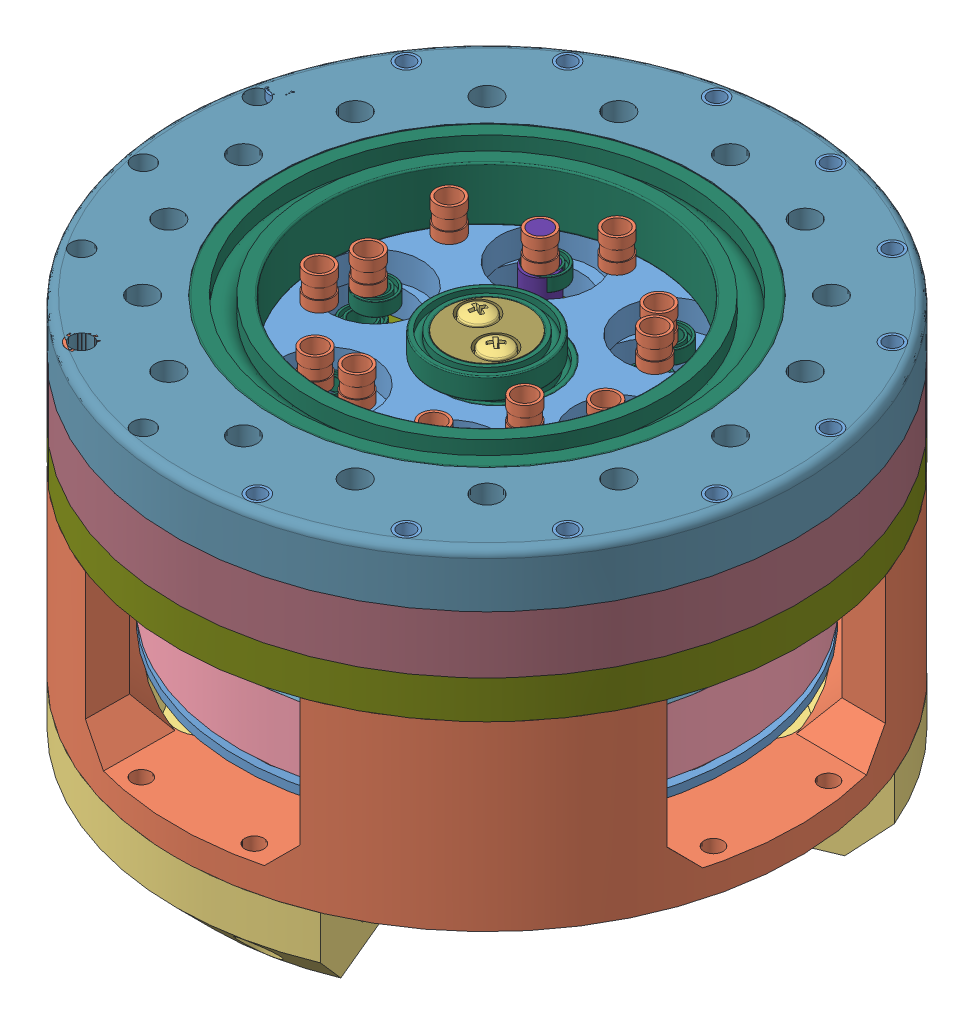
SolidWorks assembly Cycloidal, configuration Default. Lengths in mm. (continued)
Components (placement in the parent): (continued)
- hex nut style 1 gradeab_iso-1: hex nut style 1 gradeab_iso [ISO - 4032 - M3 - W - N] at (47.543 33.6573 58.7543) x (1 0 0) z (0 -1 0) size (5.5 6.35 2.4)
- Cycloidal_Discs_8308-1: Cycloidal_Discs_8308 [Default] at (106.6366 42.127 50.4062) x (-0.015094 0 0.999886) z (-0.999886 0 -0.015094) size (79.25 5 79.73)
  - Cycloidal_Discs-1: Cycloidal_Discs [Default] at (38.3081 39.5303 58.0959) size (79.25 5 79.73)
  - radial ball bearing_68_iso-1: radial ball bearing_68_iso [ISO 15 RBB - 274 - 14,SI,NC,14_68] at (18.3896 43.2803 46.5959) x (0 1 0) z (0 0 1) size (2.5 7 7)
  - radial ball bearing_68_iso-2: radial ball bearing_68_iso [ISO 15 RBB - 274 - 14,SI,NC,14_68] at (38.3081 43.2803 81.0959) x (0 1 0) z (0 0 1) size (2.5 7 7)
  - radial ball bearing_68_iso-3: radial ball bearing_68_iso [ISO 15 RBB - 274 - 14,SI,NC,14_68] at (18.3896 43.2803 69.5959) x (0 1 0) z (0 0 1) size (2.5 7 7)
  - radial ball bearing_68_iso-4: radial ball bearing_68_iso [ISO 15 RBB - 274 - 14,SI,NC,14_68] at (38.3081 43.2803 35.0959) x (0 1 0) z (0 0 1) size (2.5 7 7)
  - radial ball bearing_68_iso-5: radial ball bearing_68_iso [ISO 15 RBB - 274 - 14,SI,NC,14_68] at (58.2267 43.2803 69.5959) x (0 1 0) z (0 0 1) size (2.5 7 7)
  - radial ball bearing_68_iso-6: radial ball bearing_68_iso [ISO 15 RBB - 274 - 14,SI,NC,14_68] at (58.2267 43.2803 46.5959) x (0 1 0) z (0 0 1) size (2.5 7 7)
- Cycloidal_Discs_8308-2: Cycloidal_Discs_8308 [Default] at (106.2008 37.127 126.3479) x (-0.902001 0 0.431733) z (-0.431733 0 -0.902001) size (79.25 5 79.73)
  - Cycloidal_Discs-1: Cycloidal_Discs [Default] at (38.3081 39.5303 58.0959) size (79.25 5 79.73)
  - radial ball bearing_68_iso-1: radial ball bearing_68_iso [ISO 15 RBB - 274 - 14,SI,NC,14_68] at (18.3896 43.2803 46.5959) x (0 1 0) z (0 0 1) size (2.5 7 7)
  - radial ball bearing_68_iso-2: radial ball bearing_68_iso [ISO 15 RBB - 274 - 14,SI,NC,14_68] at (38.3081 43.2803 81.0959) x (0 1 0) z (0 0 1) size (2.5 7 7)
  - radial ball bearing_68_iso-3: radial ball bearing_68_iso [ISO 15 RBB - 274 - 14,SI,NC,14_68] at (18.3896 43.2803 69.5959) x (0 1 0) z (0 0 1) size (2.5 7 7)
  - radial ball bearing_68_iso-4: radial ball bearing_68_iso [ISO 15 RBB - 274 - 14,SI,NC,14_68] at (38.3081 43.2803 35.0959) x (0 1 0) z (0 0 1) size (2.5 7 7)
  - radial ball bearing_68_iso-5: radial ball bearing_68_iso [ISO 15 RBB - 274 - 14,SI,NC,14_68] at (58.2267 43.2803 69.5959) x (0 1 0) z (0 0 1) size (2.5 7 7)
  - radial ball bearing_68_iso-6: radial ball bearing_68_iso [ISO 15 RBB - 274 - 14,SI,NC,14_68] at (58.2267 43.2803 46.5959) x (0 1 0) z (0 0 1) size (2.5 7 7)
- m6-1: m6 [Default] at (36.6817 92.633 68.7393) x (0 0 -1) z (-1 0 0) size (6 16 6)
- Motor_Cover_v2-2: Motor_Cover_v2 [Default] at (47.267 36.0573 89.1587) x (0.999959 0 0.009078) z (-0.009078 0 0.999959) size (115 33.6 115)
- driver_cover-1: driver_cover [Default] at (47.267 36.0573 89.1587) x (0.925706 0 0.378243) z (0.378243 0 -0.925706) size (81.32 15 115)
Mates (geometry in assembly coordinates):
- Coincident1: coincident anti-aligned: plane of motor-X83008S.stp-1/outrunner.stp-1 through (63.4159 69.6573 58.6716) normal (0 1 0); plane of Base_Plate-1 through (47.267 69.6573 89.1587) normal (0 -1 0)
- Concentric1: concentric anti-aligned: line of motor-X83008S.stp-1/outrunner.stp-1 through (54.5223 64.1573 75.4616) axis (0 1 0); cylinder of Base_Plate-1 through (54.5223 76.6573 75.4616) axis (0 -1 0) radius 1.5
- Concentric2: concentric anti-aligned: cylinder of motor-X83008S.stp-1/shaft.stp-1 through (47.267 69.6573 89.1587) axis (0 1 0) radius 1.5; line of Base_Plate-1 through (47.267 76.6573 89.1587) axis (0 -1 0)
- Coincident2: coincident anti-aligned: plane of Base_Plate-1 through (47.267 76.6573 89.1587) normal (0 1 0); plane of Eccentric_Shaft-1/Eccentric_Shaft_bot-1 through (46.5649 76.6573 90.4842) normal (0 -1 0)
- Concentric75: concentric anti-aligned: cylinder of Output_Shaft-1 through (47.267 97.2573 89.1587) axis (0 -1 0) radius 30; cylinder of radial ball bearing_68_iso-39 through (47.267 71.6198 89.1587) axis (0 1 0) radius 30
- Concentric76: concentric anti-aligned: cylinder of Cover-1 through (47.267 97.2573 89.1587) axis (0 -1 0) radius 39; cylinder of radial ball bearing_68_iso-39 through (47.267 71.6198 89.1587) axis (0 1 0) radius 39
- Coincident104: coincident aligned: plane of Cover-1 through (47.267 97.2573 89.1587) normal (0 1 0); plane of radial ball bearing_68_iso-39 through (8.567 97.2573 89.1587) normal (0 1 0)
- Coincident105: coincident aligned: plane of Output_Shaft-1 through (47.267 97.2573 89.1587) normal (0 1 0); plane of Cover-1 through (47.267 97.2573 89.1587) normal (0 1 0)
- Concentric78: concentric anti-aligned: cylinder of Base_Plate-1 through (47.267 76.6573 89.1587) axis (0 -1 0) radius 20; cylinder of radial ball bearing_68_iso-40 through (47.267 52.3198 89.1587) axis (0 1 0) radius 20
- Concentric79: concentric aligned: cylinder of Ring_Pin_Housing-1 through (2.3676 87.2573 59.1579) axis (0 -1 0) radius 1.6; cylinder of Base_plate_2-1 through (2.3676 76.6573 59.1579) axis (0 -1 0) radius 1.75
- Concentric80: concentric aligned: cylinder of Ring_Pin_Housing-1 through (47.267 87.2573 89.1587) axis (0 -1 0) radius 57.5; cylinder of Base_plate_2-1 through (47.267 76.6573 89.1587) axis (0 -1 0) radius 57.5
- Coincident107: coincident anti-aligned: plane of Ring_Pin_Housing-1 through (47.267 76.6573 89.1587) normal (0 -1 0); plane of Base_plate_2-1 through (47.267 76.6573 89.1587) normal (0 1 0)
- Concentric83: concentric aligned: cylinder of Ring_Pin_Housing-1 through (2.3676 87.2573 59.1579) axis (0 -1 0) radius 1.6; cylinder of Cover-1 through (2.3676 97.2573 59.1579) axis (0 -1 0) radius 2
- Concentric84: concentric aligned: cylinder of Cover-1 through (15.4472 87.2573 57.3389) axis (0 1 0) radius 2.5; cylinder of m13_bearing-1/m6-1 through (15.4472 86.8573 57.3389) axis (0 1 0) radius 2
- Concentric85: concentric aligned: cylinder of Cover-1 through (47.267 87.2573 134.1587) axis (0 1 0) radius 2.5; cylinder of m13_bearing-11/m6-1 through (47.267 86.8573 134.1587) axis (0 1 0) radius 2
- Concentric86: concentric aligned: cylinder of Cover-1 through (64.4877 87.2573 130.7332) axis (0 1 0) radius 2.5; cylinder of m13_bearing-2/m6-1 through (64.4877 86.8573 130.7332) axis (0 1 0) radius 2
- Concentric87: concentric aligned: cylinder of Cover-1 through (79.0868 87.2573 120.9785) axis (0 1 0) radius 2.5; cylinder of m13_bearing-12/m6-1 through (79.0868 86.8573 120.9785) axis (0 1 0) radius 2
- Concentric88: concentric aligned: cylinder of Cover-1 through (88.8416 87.2573 106.3794) axis (0 1 0) radius 2.5; cylinder of m13_bearing-5/m6-1 through (88.8416 86.8573 106.3794) axis (0 1 0) radius 2
- Concentric89: concentric aligned: cylinder of Cover-1 through (92.267 87.2573 89.1587) axis (0 1 0) radius 2.5; cylinder of m13_bearing-4/m6-1 through (92.267 86.8573 89.1587) axis (0 1 0) radius 2
- Concentric90: concentric aligned: cylinder of Cover-1 through (30.0462 87.2573 47.5841) axis (0 1 0) radius 2.5; cylinder of m13_bearing-6/m6-1 through (30.0462 86.8573 47.5841) axis (0 1 0) radius 2
- Concentric91: concentric aligned: cylinder of Cover-1 through (47.267 87.2573 44.1587) axis (0 1 0) radius 2.5; cylinder of m13_bearing-3/m6-1 through (47.267 86.8573 44.1587) axis (0 1 0) radius 2
- Concentric92: concentric aligned: cylinder of Cover-1 through (64.4877 87.2573 47.5841) axis (0 1 0) radius 2.5; cylinder of m13_bearing-7/m6-1 through (64.4877 86.8573 47.5841) axis (0 1 0) radius 2
- Concentric93: concentric aligned: cylinder of Cover-1 through (79.0868 87.2573 57.3389) axis (0 1 0) radius 2.5; cylinder of m13_bearing-8/m6-1 through (79.0868 86.8573 57.3389) axis (0 1 0) radius 2
- Concentric94: concentric aligned: cylinder of Cover-1 through (88.8416 87.2573 71.9379) axis (0 1 0) radius 2.5; cylinder of m13_bearing-9/m6-1 through (88.8416 86.8573 71.9379) axis (0 1 0) radius 2
- Concentric96: concentric aligned: cylinder of Base_plate_2-1 through (47.267 76.6573 134.1587) axis (0 -1 0) radius 2.5; cylinder of socket button head screw_iso-2 through (47.267 67.4573 134.1587) axis (0 -1 0) radius 2
- Coincident121: coincident anti-aligned: plane of Base_plate_2-1 through (47.267 69.6573 89.1587) normal (0 -1 0); plane of socket button head screw_iso-2 through (45.8877 69.6573 132.7104) normal (0 1 0)
- Concentric971: concentric aligned: cylinder of Base_plate_2-1 through (15.4472 76.6573 57.3389) axis (0 -1 0) radius 2.5; cylinder of socket button head screw_iso-3 through (15.4472 67.4573 57.3389) axis (0 -1 0) radius 3.8
- Coincident1221: coincident anti-aligned: plane of Base_plate_2-1 through (47.267 69.6573 89.1587) normal (0 -1 0); plane of socket button head screw_iso-3 through (14.0679 69.6573 55.8906) normal (0 1 0)
- Concentric981: concentric aligned: cylinder of Base_plate_2-1 through (30.0462 76.6573 47.5841) axis (0 -1 0) radius 2.5; cylinder of socket button head screw_iso-4 through (30.0462 67.4573 47.5841) axis (0 -1 0) radius 3.8
- Coincident1231: coincident anti-aligned: plane of Base_plate_2-1 through (47.267 69.6573 89.1587) normal (0 -1 0); plane of socket button head screw_iso-4 through (28.6669 69.6573 46.1358) normal (0 1 0)
- Concentric991: concentric aligned: cylinder of Base_plate_2-1 through (47.267 76.6573 44.1587) axis (0 -1 0) radius 2.5; cylinder of socket button head screw_iso-5 through (47.267 67.4573 44.1587) axis (0 -1 0) radius 3.8
- Coincident1241: coincident anti-aligned: plane of Base_plate_2-1 through (47.267 69.6573 89.1587) normal (0 -1 0); plane of socket button head screw_iso-5 through (45.8877 69.6573 42.7104) normal (0 1 0)
- Concentric1001: concentric aligned: cylinder of Base_plate_2-1 through (64.4877 76.6573 47.5841) axis (0 -1 0) radius 2.5; cylinder of socket button head screw_iso-6 through (64.4877 67.4573 47.5841) axis (0 -1 0) radius 3.8
- Coincident1251: coincident anti-aligned: plane of Base_plate_2-1 through (47.267 69.6573 89.1587) normal (0 -1 0); plane of socket button head screw_iso-6 through (63.1085 69.6573 46.1358) normal (0 1 0)
- Concentric1021: concentric aligned: cylinder of Base_plate_2-1 through (88.8416 76.6573 71.9379) axis (0 -1 0) radius 2.5; cylinder of socket button head screw_iso-8 through (88.8416 67.4573 71.9379) axis (0 -1 0) radius 3.8
- Coincident1271: coincident anti-aligned: plane of Base_plate_2-1 through (47.267 69.6573 89.1587) normal (0 -1 0); plane of socket button head screw_iso-8 through (87.4623 69.6573 70.4896) normal (0 1 0)
- Concentric1031: concentric aligned: cylinder of Base_plate_2-1 through (92.267 76.6573 89.1587) axis (0 -1 0) radius 2.5; cylinder of socket button head screw_iso-9 through (92.267 67.4573 89.1587) axis (0 -1 0) radius 3.8
- Coincident1281: coincident anti-aligned: plane of Base_plate_2-1 through (47.267 69.6573 89.1587) normal (0 -1 0); plane of socket button head screw_iso-9 through (90.8877 69.6573 87.7104) normal (0 1 0)
- Concentric1041: concentric aligned: cylinder of Base_plate_2-1 through (88.8416 76.6573 106.3794) axis (0 -1 0) radius 2.5; cylinder of socket button head screw_iso-10 through (88.8416 67.4573 106.3794) axis (0 -1 0) radius 3.8
- Coincident1291: coincident anti-aligned: plane of Base_plate_2-1 through (47.267 69.6573 89.1587) normal (0 -1 0); plane of socket button head screw_iso-10 through (87.4623 69.6573 104.9311) normal (0 1 0)
- Concentric1051: concentric aligned: cylinder of Base_plate_2-1 through (79.0868 76.6573 120.9785) axis (0 -1 0) radius 2.5; cylinder of socket button head screw_iso-11 through (79.0868 67.4573 120.9785) axis (0 -1 0) radius 3.8
- Coincident1301: coincident anti-aligned: plane of Base_plate_2-1 through (47.267 69.6573 89.1587) normal (0 -1 0); plane of socket button head screw_iso-11 through (77.7075 69.6573 119.5302) normal (0 1 0)
- Coincident132: coincident anti-aligned: plane of Ring_Pin_Housing-1 through (47.267 87.2573 89.1587) normal (0 1 0); plane of Cover-1 through (47.267 87.2573 89.1587) normal (0 -1 0)
- Concentric118: concentric anti-aligned: cylinder of Output_Shaft-1 through (70.2433 97.2573 90.2013) axis (0 -1 0) radius 2.5; cylinder of M4x6x5.5_brass_insert-1 through (70.2433 86.633 90.2013) axis (0 1 0) radius 2
- Coincident144: coincident aligned: plane of Cover-1 through (47.267 97.2573 89.1587) normal (0 1 0); plane of M3x4x4.2_brass_insert-1 through (-2.9238 97.2573 74.8329) normal (0 1 0)
- Concentric1211: concentric aligned: cylinder of Cover-1 through (2.3676 97.2573 59.1579) axis (0 -1 0) radius 2; cylinder of M3x4x4.2_brass_insert-2 through (2.3676 92.3553 59.1579) axis (0 -1 0) radius 1.5
- Concentric1221: concentric aligned: cylinder of Cover-1 through (17.2662 97.2573 44.2593) axis (0 -1 0) radius 2; cylinder of M3x4x4.2_brass_insert-3 through (17.2662 92.3553 44.2593) axis (0 -1 0) radius 1.5
- Concentric1251: concentric aligned: cylinder of Cover-1 through (77.2678 97.2573 44.2593) axis (0 -1 0) radius 2; cylinder of M3x4x4.2_brass_insert-6 through (77.2678 92.3553 44.2593) axis (0 -1 0) radius 1.8
- Concentric1271: concentric anti-aligned: cylinder of Cover-1 through (100.2294 97.2573 78.6238) axis (0 -1 0) radius 2; cylinder of M3x4x4.2_brass_insert-8 through (100.2294 98.1594 78.6238) axis (0 1 0) radius 1.8
- Concentric1331: concentric aligned: cylinder of Cover-1 through (36.7321 97.2573 36.1963) axis (0 -1 0) radius 2; cylinder of M3x4x4.2_brass_insert-14 through (36.7321 92.3553 36.1963) axis (0 -1 0) radius 1.8
- Concentric1341: concentric anti-aligned: cylinder of Cover-1 through (57.8019 97.2573 36.1963) axis (0 -1 0) radius 2; cylinder of M3x4x4.2_brass_insert-15 through (57.8019 98.1594 36.1963) axis (0 1 0) radius 2
- Concentric1351: concentric aligned: cylinder of Cover-1 through (92.1663 97.2573 59.1579) axis (0 -1 0) radius 2; cylinder of M3x4x4.2_brass_insert-16 through (92.1663 92.3553 59.1579) axis (0 -1 0) radius 2
- Concentric1361: concentric aligned: cylinder of Cover-1 through (100.2294 97.2573 99.6935) axis (0 -1 0) radius 2; cylinder of M3x4x4.2_brass_insert-17 through (100.2294 92.3553 99.6935) axis (0 -1 0) radius 2
- Concentric1381: concentric aligned: cylinder of Cover-1 through (92.1663 97.2573 119.1595) axis (0 -1 0) radius 2; cylinder of M3x4x4.2_brass_insert-19 through (92.1663 92.3553 119.1595) axis (0 -1 0) radius 2
- Concentric1391: concentric aligned: cylinder of Cover-1 through (77.2678 97.2573 134.058) axis (0 -1 0) radius 2; cylinder of M3x4x4.2_brass_insert-20 through (77.2678 92.3553 134.058) axis (0 -1 0) radius 1.5
- Concentric1401: concentric aligned: cylinder of Cover-1 through (57.8019 97.2573 142.1211) axis (0 -1 0) radius 2; cylinder of M3x4x4.2_brass_insert-21 through (57.8019 92.3553 142.1211) axis (0 -1 0) radius 1.5
- Coincident205: coincident aligned: plane of M3x4x4.2_brass_insert-1 through (-2.9238 97.2573 74.8329) normal (0 1 0); plane of M3x4x4.2_brass_insert-2 through (1.3472 97.2573 58.0584) normal (0 1 0)
- Coincident206: coincident aligned: plane of M3x4x4.2_brass_insert-1 through (-2.9238 97.2573 74.8329) normal (0 1 0); plane of M3x4x4.2_brass_insert-3 through (16.5019 97.2573 42.9686) normal (0 1 0)
- Coincident207: coincident aligned: plane of M3x4x4.2_brass_insert-1 through (-2.9238 97.2573 74.8329) normal (0 1 0); plane of M3x4x4.2_brass_insert-14 through (37.4964 97.2573 37.4869) normal (0 1 0)
- Coincident208: coincident aligned: plane of M3x4x4.2_brass_insert-1 through (-2.9238 97.2573 74.8329) normal (0 1 0); plane of M3x4x4.2_brass_insert-15 through (59.5962 97.2573 35.313) normal (0 1 0)
- Coincident209: coincident aligned: plane of M3x4x4.2_brass_insert-1 through (-2.9238 97.2573 74.8329) normal (0 1 0); plane of M3x4x4.2_brass_insert-6 through (76.2474 97.2573 43.1599) normal (0 1 0)
- Coincident210: coincident aligned: plane of M3x4x4.2_brass_insert-1 through (-2.9238 97.2573 74.8329) normal (0 1 0); plane of M3x4x4.2_brass_insert-16 through (91.1459 97.2573 58.0584) normal (0 1 0)
- Coincident211: coincident aligned: plane of M3x4x4.2_brass_insert-1 through (-2.9238 97.2573 74.8329) normal (0 1 0); plane of M3x4x4.2_brass_insert-8 through (98.2886 97.2573 79.1069) normal (0 1 0)
- Coincident212: coincident aligned: plane of M3x4x4.2_brass_insert-1 through (-2.9238 97.2573 74.8329) normal (0 1 0); plane of M3x4x4.2_brass_insert-17 through (101.2498 97.2573 100.793) normal (0 1 0)
- Coincident213: coincident aligned: plane of M3x4x4.2_brass_insert-1 through (-2.9238 97.2573 74.8329) normal (0 1 0); plane of M3x4x4.2_brass_insert-19 through (93.1868 97.2573 120.2589) normal (0 1 0)
- Coincident214: coincident aligned: plane of M3x4x4.2_brass_insert-1 through (-2.9238 97.2573 74.8329) normal (0 1 0); plane of M3x4x4.2_brass_insert-20 through (78.2882 97.2573 135.1575) normal (0 1 0)
- Coincident215: coincident aligned: plane of M3x4x4.2_brass_insert-1 through (-2.9238 97.2573 74.8329) normal (0 1 0); plane of M3x4x4.2_brass_insert-21 through (58.8223 97.2573 143.2205) normal (0 1 0)
- Concentric14021: concentric aligned: cylinder of Output_Shaft-1 through (34.8759 97.2573 108.5355) axis (0 -1 0) radius 2.5; cylinder of M4x6x5.5_brass_insert-4 through (34.8759 80.689 108.5355) axis (0 -1 0) radius 2.5
- Concentric14031: concentric aligned: cylinder of Output_Shaft-1 through (24.2906 97.2573 88.1161) axis (0 -1 0) radius 2.5; cylinder of M4x6x5.5_brass_insert-5 through (24.2906 80.689 88.1161) axis (0 -1 0) radius 2.5
- Concentric14041: concentric aligned: cylinder of Output_Shaft-1 through (36.6817 97.2573 68.7393) axis (0 -1 0) radius 2.5; cylinder of M4x6x5.5_brass_insert-6 through (36.6817 80.689 68.7393) axis (0 -1 0) radius 2.5
- Concentric14051: concentric aligned: cylinder of Output_Shaft-1 through (59.6581 97.2573 69.7819) axis (0 -1 0) radius 2.5; cylinder of M4x6x5.5_brass_insert-7 through (59.6581 80.689 69.7819) axis (0 -1 0) radius 2.5
- Concentric14061: concentric aligned: cylinder of Output_Shaft-1 through (66.6438 97.2573 101.5498) axis (0 -1 0) radius 2.5; cylinder of M4x6x5.5_brass_insert-8 through (66.6438 85.3133 101.5498) axis (0 -1 0) radius 2.5
- Concentric14071: concentric aligned: cylinder of Output_Shaft-1 through (67.6864 97.2573 78.5734) axis (0 -1 0) radius 2.5; cylinder of M4x6x5.5_brass_insert-9 through (67.6864 85.3133 78.5734) axis (0 -1 0) radius 2.5
- Concentric14081: concentric aligned: cylinder of Output_Shaft-1 through (48.3096 97.2573 66.1823) axis (0 -1 0) radius 2.5; cylinder of M4x6x5.5_brass_insert-10 through (48.3096 85.3133 66.1823) axis (0 -1 0) radius 2.5
- Concentric14091: concentric aligned: cylinder of Output_Shaft-1 through (27.8902 97.2573 76.7676) axis (0 -1 0) radius 2.5; cylinder of M4x6x5.5_brass_insert-11 through (27.8902 85.3133 76.7676) axis (0 -1 0) radius 2.5
- Concentric14111: concentric aligned: cylinder of Output_Shaft-1 through (26.8476 97.2573 99.7439) axis (0 -1 0) radius 2.5; cylinder of M4x6x5.5_brass_insert-13 through (26.8476 85.3133 99.7439) axis (0 -1 0) radius 2.5
- Concentric14121: concentric aligned: cylinder of Output_Shaft-1 through (46.2244 97.2573 112.135) axis (0 -1 0) radius 2.5; cylinder of M4x6x5.5_brass_insert-14 through (46.2244 85.3133 112.135) axis (0 -1 0) radius 2.5
- Concentric14131: concentric aligned: cylinder of Output_Shaft-1 through (57.8522 97.2573 109.5781) axis (0 -1 0) radius 2.5; cylinder of M4x6x5.5_brass_insert-15 through (57.8522 80.689 109.5781) axis (0 -1 0) radius 2.5
- Coincident1435: coincident aligned: plane of M4x6x5.5_brass_insert-1 through (68.3788 92.633 91.8666) normal (0 1 0); plane of M4x6x5.5_brass_insert-15 through (57.8522 92.633 109.5781) normal (0 1 0)
- Coincident1436: coincident aligned: plane of M4x6x5.5_brass_insert-1 through (68.3788 92.633 91.8666) normal (0 1 0); plane of M4x6x5.5_brass_insert-4 through (34.8759 92.633 108.5355) normal (0 1 0)
- Coincident1437: coincident aligned: plane of M4x6x5.5_brass_insert-1 through (68.3788 92.633 91.8666) normal (0 1 0); plane of M4x6x5.5_brass_insert-5 through (24.2906 92.633 88.1161) normal (0 1 0)
- Coincident1438: coincident aligned: plane of M4x6x5.5_brass_insert-1 through (68.3788 92.633 91.8666) normal (0 1 0); plane of M4x6x5.5_brass_insert-6 through (36.6817 92.633 68.7393) normal (0 1 0)
- Coincident1439: coincident aligned: plane of M4x6x5.5_brass_insert-1 through (68.3788 92.633 91.8666) normal (0 1 0); plane of M4x6x5.5_brass_insert-7 through (59.6581 92.633 69.7819) normal (0 1 0)
- Coincident1440: coincident aligned: plane of Output_Shaft-1 through (47.267 97.2573 89.1587) normal (0 1 0); plane of M4x6x5.5_brass_insert-9 through (67.6864 97.2573 78.5734) normal (0 1 0)
- Coincident1441: coincident aligned: plane of Output_Shaft-1 through (47.267 97.2573 89.1587) normal (0 1 0); plane of M4x6x5.5_brass_insert-8 through (66.6438 97.2573 101.5498) normal (0 1 0)
- Coincident1442: coincident aligned: plane of Output_Shaft-1 through (47.267 97.2573 89.1587) normal (0 1 0); plane of M4x6x5.5_brass_insert-14 through (46.2244 97.2573 112.135) normal (0 1 0)
- Coincident1443: coincident aligned: plane of Output_Shaft-1 through (47.267 97.2573 89.1587) normal (0 1 0); plane of M4x6x5.5_brass_insert-13 through (26.8476 97.2573 99.7439) normal (0 1 0)
- Coincident1444: coincident aligned: plane of Output_Shaft-1 through (47.267 97.2573 89.1587) normal (0 1 0); plane of M4x6x5.5_brass_insert-11 through (27.8902 97.2573 76.7676) normal (0 1 0)
- Coincident1445: coincident aligned: plane of Output_Shaft-1 through (47.267 97.2573 89.1587) normal (0 1 0); plane of M4x6x5.5_brass_insert-10 through (48.3096 97.2573 66.1823) normal (0 1 0)
- Concentric14151: concentric aligned: cylinder of m13_bearing-2/m6-1 through (64.4877 86.8573 130.7332) axis (0 1 0) radius 2; cylinder of M4x6x5.5_brass_insert-20 through (64.4877 86.8573 130.7332) axis (0 1 0) radius 2
- Concentric14161: concentric aligned: cylinder of m13_bearing-11/m6-1 through (47.267 86.8573 134.1587) axis (0 1 0) radius 2; cylinder of M4x6x5.5_brass_insert-21 through (47.267 86.8573 134.1587) axis (0 1 0) radius 2
- Concentric14171: concentric aligned: cylinder of m13_bearing-1/m6-1 through (15.4472 86.8573 57.3389) axis (0 1 0) radius 2; cylinder of M4x6x5.5_brass_insert-22 through (15.4472 86.8573 57.3389) axis (0 1 0) radius 2
- Concentric14181: concentric aligned: cylinder of m13_bearing-6/m6-1 through (30.0462 86.8573 47.5841) axis (0 1 0) radius 2; cylinder of M4x6x5.5_brass_insert-23 through (30.0462 86.8573 47.5841) axis (0 1 0) radius 2
- Concentric14191: concentric aligned: cylinder of m13_bearing-12/m6-1 through (79.0868 86.8573 120.9785) axis (0 1 0) radius 2; cylinder of M4x6x5.5_brass_insert-24 through (79.0868 98.8014 120.9785) axis (0 1 0) radius 2.3
- Concentric14201: concentric aligned: cylinder of m13_bearing-5/m6-1 through (88.8416 86.8573 106.3794) axis (0 1 0) radius 2; cylinder of M4x6x5.5_brass_insert-25 through (88.8416 86.8573 106.3794) axis (0 1 0) radius 2
- Concentric14211: concentric aligned: cylinder of m13_bearing-4/m6-1 through (92.267 86.8573 89.1587) axis (0 1 0) radius 2; cylinder of M4x6x5.5_brass_insert-26 through (92.267 86.8573 89.1587) axis (0 1 0) radius 2
- Concentric14221: concentric aligned: cylinder of m13_bearing-9/m6-1 through (88.8416 86.8573 71.9379) axis (0 1 0) radius 2; cylinder of M4x6x5.5_brass_insert-27 through (88.8416 86.8573 71.9379) axis (0 1 0) radius 2
- Concentric14231: concentric aligned: line of Ring_Pin_Housing-1 through (79.0868 87.2573 57.3389) axis (0 -1 0); cylinder of M4x6x5.5_brass_insert-28 through (79.0868 92.8573 57.3389) axis (0 -1 0) radius 2
- Concentric14241: concentric aligned: cylinder of m13_bearing-7/m6-1 through (64.4877 86.8573 47.5841) axis (0 1 0) radius 2; cylinder of M4x6x5.5_brass_insert-29 through (64.4877 86.8573 47.5841) axis (0 1 0) radius 2
- Concentric14251: concentric aligned: cylinder of m13_bearing-3/m6-1 through (47.267 86.8573 44.1587) axis (0 1 0) radius 2; cylinder of M4x6x5.5_brass_insert-31 through (47.267 86.8573 44.1587) axis (0 1 0) radius 2
- Coincident1447: coincident anti-aligned: plane of m13_bearing-2/m6-1 through (64.4877 86.8573 130.7332) normal (0 1 0); plane of M4x6x5.5_brass_insert-20 through (64.4877 86.8573 130.7332) normal (0 -1 0)
- Coincident1458: coincident aligned: plane of M4x6x5.5_brass_insert-20 through (62.6232 92.8573 132.3986) normal (0 1 0); plane of M4x6x5.5_brass_insert-21 through (45.4024 92.8573 135.824) normal (0 1 0)
- Coincident1459: coincident aligned: plane of M4x6x5.5_brass_insert-20 through (62.6232 92.8573 132.3986) normal (0 1 0); plane of M4x6x5.5_brass_insert-22 through (17.0054 92.8573 59.2938) normal (0 1 0)
- Coincident1460: coincident aligned: plane of M4x6x5.5_brass_insert-20 through (62.6232 92.8573 132.3986) normal (0 1 0); plane of M4x6x5.5_brass_insert-23 through (31.6045 92.8573 49.5391) normal (0 1 0)
- Coincident1461: coincident aligned: plane of M4x6x5.5_brass_insert-20 through (62.6232 92.8573 132.3986) normal (0 1 0); plane of M4x6x5.5_brass_insert-31 through (46.7161 92.8573 46.5972) normal (0 1 0)
- Coincident1462: coincident aligned: plane of M4x6x5.5_brass_insert-20 through (62.6232 92.8573 132.3986) normal (0 1 0); plane of M4x6x5.5_brass_insert-29 through (64.1304 92.8573 50.0584) normal (0 1 0)
- Coincident1463: coincident aligned: plane of M4x6x5.5_brass_insert-20 through (62.6232 92.8573 132.3986) normal (0 1 0); plane of M4x6x5.5_brass_insert-28 through (79.0868 92.8573 57.3389) normal (0 1 0)
- Coincident1464: coincident aligned: plane of M4x6x5.5_brass_insert-20 through (62.6232 92.8573 132.3986) normal (0 1 0); plane of M4x6x5.5_brass_insert-27 through (86.977 92.8573 73.6032) normal (0 1 0)
- Coincident1465: coincident aligned: plane of M4x6x5.5_brass_insert-20 through (62.6232 92.8573 132.3986) normal (0 1 0); plane of M4x6x5.5_brass_insert-26 through (90.4024 92.8573 90.824) normal (0 1 0)
- Coincident1466: coincident aligned: plane of M4x6x5.5_brass_insert-20 through (62.6232 92.8573 132.3986) normal (0 1 0); plane of M4x6x5.5_brass_insert-25 through (86.977 92.8573 108.0448) normal (0 1 0)
- Coincident1467: coincident aligned: plane of M4x6x5.5_brass_insert-20 through (62.6232 92.8573 132.3986) normal (0 1 0); plane of M4x6x5.5_brass_insert-24 through (80.4417 92.8573 123.0795) normal (0 1 0)
- Concentric1426: concentric aligned: cylinder of pan cross head_am-1 through (50.8017 117.9573 91.031) axis (0 1 0) radius 1.5; line of Eccentric_Shaft-1/Eccentric_Shaft_top-1 through (50.8017 90.1573 91.031) axis (0 1 0)
- Coincident1468: coincident anti-aligned: plane of Eccentric_Shaft-1/Eccentric_Shaft_top-1 through (43.7323 90.1573 87.2863) normal (0 1 0); plane of pan cross head_am-1 through (51.7959 90.1573 89.9078) normal (0 -1 0)
- Concentric14281: concentric aligned: cylinder of pan cross head_am-3 through (43.7323 117.9573 87.2863) axis (0 1 0) radius 2.8; cylinder of Eccentric_Shaft-1/Eccentric_Shaft_top-1 through (43.7323 86.6573 87.2863) axis (0 1 0) radius 1.5
- Coincident14701: coincident anti-aligned: plane of Eccentric_Shaft-1/Eccentric_Shaft_top-1 through (50.8017 90.1573 91.031) normal (0 1 0); plane of pan cross head_am-3 through (44.2427 90.1573 85.8758) normal (0 -1 0)
- Concentric1437: concentric anti-aligned: cylinder of Base_Plate-1 through (50.8017 76.6573 91.031) axis (0 -1 0) radius 2; cylinder of M3x4x4.2_brass_insert-22 through (50.8017 74.5594 91.031) axis (0 1 0) radius 1.5
- Coincident1479: coincident aligned: plane of Base_Plate-1 through (47.267 69.6573 89.1587) normal (0 -1 0); plane of M3x4x4.2_brass_insert-22 through (52.2786 69.6573 90.7689) normal (0 -1 0)
- Concentric1438: concentric anti-aligned: cylinder of Base_Plate-1 through (43.7323 76.6573 87.2863) axis (0 -1 0) radius 2; cylinder of M3x4x4.2_brass_insert-23 through (43.7323 74.5594 87.2863) axis (0 1 0) radius 1.5
- Coincident1480: coincident aligned: plane of Base_Plate-1 through (47.267 69.6573 89.1587) normal (0 -1 0); plane of M3x4x4.2_brass_insert-23 through (45.2092 69.6573 87.0242) normal (0 -1 0)
- Concentric1439: concentric anti-aligned: cylinder of Base_Plate-1 through (33.5699 76.6573 81.9033) axis (0 -1 0) radius 1.5; cylinder of pan cross head_am-4 through (33.5699 102.9573 81.9033) axis (0 1 0) radius 1.5
- Coincident1481: coincident anti-aligned: plane of Base_Plate-1 through (33.5699 75.1573 81.9033) normal (0 1 0); plane of pan cross head_am-4 through (35.0699 75.1573 81.9033) normal (0 -1 0)
- Concentric14401: concentric anti-aligned: cylinder of Base_Plate-1 through (60.9641 76.6573 96.414) axis (0 -1 0) radius 1.5; cylinder of pan cross head_am-5 through (60.9641 102.9573 96.414) axis (0 1 0) radius 2.8
- Coincident14821: coincident anti-aligned: plane of Base_Plate-1 through (60.9641 75.1573 96.414) normal (0 1 0); plane of pan cross head_am-5 through (62.4641 75.1573 96.414) normal (0 -1 0)
- Concentric144131: concentric aligned: cylinder of Cover-1 through (17.2662 97.2573 134.058) axis (0 -1 0) radius 2; cylinder of M4x6x5.5_brass_insert-45 through (17.2662 97.2573 134.058) axis (0 -1 0) radius 2
- Coincident14823: coincident aligned: plane of Cover-1 through (47.267 97.2573 89.1587) normal (0 1 0); plane of M4x6x5.5_brass_insert-45 through (17.2662 97.2573 134.058) normal (0 1 0)
- GearMate1: gear = 10 : 1 mm: cylinder of Eccentric_Shaft-1/Eccentric_Shaft_top-1 through (47.267 91.6573 89.1587) axis (0 -1 0) radius 7.5; cylinder of Output_Shaft-1 through (47.267 97.2573 89.1587) axis (0 -1 0) radius 10.5
- Concentric1445021: concentric anti-aligned: cylinder of Base_Plate-1 through (40.0117 76.6573 102.8558) axis (0 -1 0) radius 1.5; cylinder of pan cross head_am-6 through (40.0117 102.9573 102.8558) axis (0 1 0) radius 2.8
- Coincident1486621: coincident anti-aligned: plane of Base_Plate-1 through (40.0117 75.1573 102.8558) normal (0 1 0); plane of pan cross head_am-6 through (41.5117 75.1573 102.8558) normal (0 -1 0)
- Concentric1445031: concentric anti-aligned: cylinder of Base_Plate-1 through (54.5223 76.6573 75.4616) axis (0 -1 0) radius 1.5; cylinder of pan cross head_am-7 through (54.5223 102.9573 75.4616) axis (0 1 0) radius 2.8
- Coincident1486631: coincident anti-aligned: plane of Base_Plate-1 through (54.5223 75.1573 75.4616) normal (0 1 0); plane of pan cross head_am-7 through (56.0223 75.1573 75.4616) normal (0 -1 0)
- Coincident1486632: coincident anti-aligned: plane of Cover-1 through (88.8416 86.8573 71.9379) normal (0 -1 0); plane of m13_bearing-9/radial ball bearing_68_iso-2 through (91.6245 86.8573 68.9955) normal (0 1 0)
- Coincident1486633: coincident anti-aligned: plane of Cover-1 through (88.8416 86.8573 71.9379) normal (0 -1 0); plane of m13_bearing-8/radial ball bearing_68_iso-2 through (78.4447 86.8573 53.3401) normal (0 1 0)
- Coincident1486634: coincident anti-aligned: plane of Cover-1 through (88.8416 86.8573 71.9379) normal (0 -1 0); plane of m13_bearing-7/radial ball bearing_68_iso-2 through (66.6983 86.8573 44.1906) normal (0 1 0)
- Coincident1486635: coincident anti-aligned: plane of Cover-1 through (88.8416 86.8573 71.9379) normal (0 -1 0); plane of m13_bearing-3/radial ball bearing_68_iso-2 through (47.4539 86.8573 40.113) normal (0 1 0)
- Coincident1486636: coincident anti-aligned: plane of Cover-1 through (88.8416 86.8573 71.9379) normal (0 -1 0); plane of m13_bearing-4/radial ball bearing_68_iso-2 through (92.1768 86.8573 85.1097) normal (0 1 0)
- Coincident1486637: coincident anti-aligned: plane of Cover-1 through (88.8416 86.8573 71.9379) normal (0 -1 0); plane of m13_bearing-5/radial ball bearing_68_iso-2 through (88.6021 86.8573 102.3365) normal (0 1 0)
- Coincident1486638: coincident anti-aligned: plane of Cover-1 through (88.8416 86.8573 71.9379) normal (0 -1 0); plane of m13_bearing-12/radial ball bearing_68_iso-2 through (78.3409 86.8573 116.9978) normal (0 1 0)
- Coincident1486639: coincident anti-aligned: plane of Cover-1 through (88.8416 86.8573 71.9379) normal (0 -1 0); plane of m13_bearing-11/radial ball bearing_68_iso-2 through (44.9443 86.8573 130.8409) normal (0 1 0)
- Coincident1486640: coincident anti-aligned: plane of Cover-1 through (88.8416 86.8573 71.9379) normal (0 -1 0); plane of m13_bearing-2/radial ball bearing_68_iso-2 through (64.0006 86.8573 126.7126) normal (0 1 0)
- Coincident1486643: coincident anti-aligned: plane of Cover-1 through (30.0462 86.8573 47.5841) normal (0 -1 0); plane of m13_bearing-6/radial ball bearing_68_iso-2 through (28.2174 86.8573 43.9705) normal (0 1 0)
- Coincident1486644: coincident anti-aligned: plane of Cover-1 through (15.4472 86.8573 57.3389) normal (0 -1 0); plane of m13_bearing-1/radial ball bearing_68_iso-2 through (12.4643 86.8573 54.5994) normal (0 1 0)
- Concentric1445035: concentric anti-aligned: cylinder of Eccentric_Shaft-1/Eccentric_Shaft_bot-1 through (46.5649 81.6573 90.4842) axis (0 -1 0) radius 7.5; cylinder of radial ball bearing_68_iso-46 through (46.5649 59.0198 90.4842) axis (0 1 0) radius 7.5
- Coincident1486648: coincident aligned: plane of Eccentric_Shaft-1/Eccentric_Shaft_bot-1 through (46.5649 81.6573 90.4842) normal (0 1 0); plane of radial ball bearing_68_iso-46 through (38.8649 81.6573 90.4842) normal (0 1 0)
- Concentric1445036: concentric anti-aligned: cylinder of Eccentric_Shaft-1/Eccentric_Shaft_bot-2 through (47.9691 86.6573 87.8331) axis (0 -1 0) radius 7.5; cylinder of radial ball bearing_68_iso-44 through (47.9691 64.0198 87.8331) axis (0 1 0) radius 7.5
- Coincident1486649: coincident aligned: plane of Eccentric_Shaft-1/Eccentric_Shaft_bot-2 through (47.9691 82.6573 87.8331) normal (0 1 0); circle of radial ball bearing_68_iso-44
- Concentric1445037: concentric anti-aligned: cylinder of Eccentric_Shaft-1/Eccentric_Shaft_top-1 through (47.267 91.6573 89.1587) axis (0 -1 0) radius 7.5; cylinder of radial ball bearing_68_iso-45 through (47.267 69.0198 89.1587) axis (0 1 0) radius 7.5
- Concentric1445038: concentric anti-aligned: cylinder of Base_Plate-1 through (47.267 76.6573 89.1587) axis (0 -1 0) radius 20; cylinder of radial ball bearing_68_iso-40 through (47.267 52.3198 89.1587) axis (0 1 0) radius 20
- Coincident1486651: coincident aligned: plane of Base_Plate-1 through (47.267 76.6573 89.1587) normal (0 1 0); plane of Base_plate_2-1 through (47.267 76.6573 89.1587) normal (0 1 0)
- Concentric1445041: concentric anti-aligned: cylinder of radial ball bearing_68_iso-40 through (47.267 52.3198 89.1587) axis (0 1 0) radius 26; cylinder of Base_plate_2-1 through (47.267 76.6573 89.1587) axis (0 -1 0) radius 26
- Coincident1486655: coincident anti-aligned: plane of Eccentric_Shaft-1/Eccentric_Shaft_top-1 through (47.267 87.6573 89.1587) normal (0 1 0); plane of radial ball bearing_68_iso-45 through (47.5372 87.6573 97.5543) normal (0 -1 0)
- Concentric1445042: concentric anti-aligned: cylinder of Base_Plate-1 through (43.7323 76.6573 87.2863) axis (0 -1 0) radius 2; cylinder of Eccentric_Shaft-1/Eccentric_Shaft_bot-1 through (43.7323 76.6573 87.2863) axis (0 1 0) radius 1.5
- Concentric1445043: concentric aligned: cylinder of Eccentric_Shaft-1/Eccentric_Shaft_bot-1 through (50.8017 76.6573 91.031) axis (0 1 0) radius 1.5; cylinder of M3x4x4.2_brass_insert-22 through (50.8017 74.5594 91.031) axis (0 1 0) radius 1.5
- Concentric1445044: concentric aligned: cylinder of Base_plate_2-1 through (79.0868 76.6573 57.3389) axis (0 -1 0) radius 2.5; cylinder of socket button head screw_iso-37 through (79.0868 67.4573 57.3389) axis (0 -1 0) radius 2
- Coincident1486656: coincident anti-aligned: plane of Base_plate_2-1 through (47.267 69.6573 89.1587) normal (0 -1 0); plane of socket button head screw_iso-37 through (77.6783 69.6573 55.9189) normal (0 1 0)
- Concentric1445045: concentric aligned: cylinder of Base_plate_2-1 through (64.4877 76.6573 130.7332) axis (0 -1 0) radius 2.5; cylinder of socket button head screw_iso-38 through (64.4877 67.4573 130.7332) axis (0 -1 0) radius 2
- Coincident1486657: coincident anti-aligned: plane of Base_plate_2-1 through (47.267 69.6573 89.1587) normal (0 -1 0); plane of socket button head screw_iso-38 through (63.1085 69.6573 129.285) normal (0 1 0)
- Coincident1486660: coincident aligned: plane of Cover-1 through (5.6924 86.8573 71.9379) normal (0 -1 0); circle of m13_bearing-31/radial ball bearing_68_iso-2
- Coincident1486661: coincident aligned: plane of Cover-1 through (5.6924 86.8573 71.9379) normal (0 -1 0); circle of m13_bearing-32/radial ball bearing_68_iso-2
- Coincident1486662: coincident aligned: plane of Cover-1 through (5.6924 86.8573 71.9379) normal (0 -1 0); circle of m13_bearing-36/radial ball bearing_68_iso-2
- Coincident1486663: coincident aligned: plane of Cover-1 through (5.6924 86.8573 71.9379) normal (0 -1 0); circle of m13_bearing-35/radial ball bearing_68_iso-2
- Coincident1486664: coincident aligned: plane of Cover-1 through (5.6924 86.8573 71.9379) normal (0 -1 0); circle of m13_bearing-34/radial ball bearing_68_iso-2
- Concentric1445052: concentric aligned: circle of m13_bearing-31/m6-1; cylinder of M4x6x5.5_brass_insert-47 through (5.6924 92.8573 71.9379) axis (0 -1 0) radius 2
- Concentric14450531: concentric aligned: line of Cover-1 through (5.6924 86.8573 106.3794) axis (0 1 0); cylinder of M4x6x5.5_brass_insert-49 through (5.6924 87.0073 106.3794) axis (0 1 0) radius 2
- Concentric14450541: concentric aligned: line of Cover-1 through (15.4472 86.8573 120.9785) axis (0 1 0); cylinder of M4x6x5.5_brass_insert-50 through (15.4472 86.8573 120.9785) axis (0 1 0) radius 2
- Concentric1445056: concentric aligned: circle of m13_bearing-32/m6-1; cylinder of M4x6x5.5_brass_insert-48 through (2.267 92.8573 89.1587) axis (0 -1 0) radius 2
- Concentric1445057: concentric aligned: cylinder of Base_plate_2-1 through (5.6924 76.6573 71.9379) axis (0 -1 0) radius 2.5; cylinder of m13_bearing-31/radial ball bearing_68_iso-2 through (5.6924 104.9948 71.9379) axis (0 -1 0) radius 6.5
- Concentric1445058: concentric aligned: cylinder of Ring_Pin_Housing-1 through (2.267 87.2573 89.1587) axis (0 -1 0) radius 7; cylinder of m13_bearing-32/radial ball bearing_68_iso-2 through (2.267 104.9948 89.1587) axis (0 -1 0) radius 6.5
- Concentric1445059: concentric aligned: cylinder of Ring_Pin_Housing-1 through (5.6924 87.2573 106.3794) axis (0 -1 0) radius 7; cylinder of m13_bearing-36/radial ball bearing_68_iso-2 through (5.6924 105.1448 106.3794) axis (0 -1 0) radius 6.5
- Concentric1445060: concentric aligned: cylinder of Ring_Pin_Housing-1 through (15.4472 87.2573 120.9785) axis (0 -1 0) radius 7; cylinder of m13_bearing-35/radial ball bearing_68_iso-2 through (15.4472 104.9948 120.9785) axis (0 -1 0) radius 6.5
- Concentric1445061: concentric aligned: cylinder of Ring_Pin_Housing-1 through (30.0462 87.2573 130.7332) axis (0 -1 0) radius 7; cylinder of m13_bearing-34/radial ball bearing_68_iso-2 through (30.0462 105.1448 130.7332) axis (0 -1 0) radius 6.5
- Coincident1486681: coincident anti-aligned: plane of m13_bearing-1/m6-1 through (15.4472 92.8573 57.3389) normal (0 1 0); circle of M4x6x5.5_brass_insert-47
- Concentric1445063: concentric aligned: cylinder of m13_bearing-34/m6-1 through (30.0462 87.0073 130.7332) axis (0 1 0) radius 2; cylinder of M4x6x5.5_brass_insert-51 through (30.0462 87.0073 130.7332) axis (0 1 0) radius 2
- Coincident1486686: coincident aligned: plane of m13_bearing-36/m6-1 through (5.6924 93.0073 106.3794) normal (0 1 0); circle of M4x6x5.5_brass_insert-49
- Coincident1486687: coincident anti-aligned: plane of m13_bearing-32/m6-1 through (2.267 92.8573 89.1587) normal (0 1 0); circle of M4x6x5.5_brass_insert-48
- Coincident1486688: coincident aligned: plane of m13_bearing-35/m6-1 through (15.4472 92.8573 120.9785) normal (0 1 0); circle of M4x6x5.5_brass_insert-50
- Coincident1486690: coincident aligned: plane of m13_bearing-34/m6-1 through (30.0462 93.0073 130.7332) normal (0 1 0); circle of M4x6x5.5_brass_insert-51
- Coincident1486692: coincident anti-aligned: plane of foc-motor-controller.step-1/foc-motor-controller_PCB.step-1 through (47.267 33.6573 89.1587) normal (0 1 0); plane of hex nut style 1 gradeab_iso-1 through (47.543 33.6573 61.9298) normal (0 -1 0)
- Concentric14450545: concentric anti-aligned: cylinder of radial ball bearing_68_iso-46 through (46.5649 59.0198 90.4842) axis (0 1 0) radius 10.5; cylinder of Cycloidal_Discs_8308-2/Cycloidal_Discs-1 through (46.5649 81.6573 90.4842) axis (0 -1 0) radius 10.5
- Coincident1486693: coincident aligned: plane of radial ball bearing_68_iso-46 through (36.2649 81.6573 90.4842) normal (0 1 0); plane of Cycloidal_Discs_8308-2/Cycloidal_Discs-1 through (62.9758 81.6573 125.1584) normal (0 1 0)
- Concentric14450546: concentric anti-aligned: cylinder of radial ball bearing_68_iso-44 through (47.9691 64.0198 87.8331) axis (0 1 0) radius 10.5; cylinder of Cycloidal_Discs_8308-1/Cycloidal_Discs-1 through (47.9691 86.6573 87.8331) axis (0 -1 0) radius 10.5
- Coincident1486694: coincident aligned: plane of radial ball bearing_68_iso-44 through (55.1706 86.6573 80.4691) normal (0 1 0); plane of Cycloidal_Discs_8308-1/Cycloidal_Discs-1 through (86.3236 86.6573 88.5794) normal (0 1 0)
- Concentric14450547: concentric anti-aligned: cylinder of M4x6x5.5_brass_insert-6 through (36.6817 92.633 68.7393) axis (0 -1 0) radius 2; cylinder of m6-1 through (36.6817 86.633 68.7393) axis (0 1 0) radius 2
- Coincident1486695: coincident anti-aligned: circle of M4x6x5.5_brass_insert-6; plane of m6-1 through (36.6817 86.633 68.7393) normal (0 1 0)
- Tangent1: tangent aligned: cylinder of Cycloidal_Discs_8308-1/radial ball bearing_68_iso-3 through (36.7711 64.7698 67.7433) axis (0 1 0) radius 2; cylinder of m6-1 through (36.6817 76.633 68.7393) axis (0 1 0) radius 3
- Tangent3: tangent aligned: cylinder of Cycloidal_Discs_8308-2/radial ball bearing_68_iso-2 through (36.635 59.7698 69.7382) axis (0 1 0) radius 2; cylinder of m6-1 through (36.6817 76.633 68.7393) axis (0 1 0) radius 3
- Concentric14450552: concentric aligned: cylinder of Ring_Pin_Housing-1 through (47.267 87.2573 89.1587) axis (0 -1 0) radius 57.5; cylinder of Cover-1 through (47.267 97.2573 89.1587) axis (0 -1 0) radius 57.5
- Concentric14450553: concentric aligned: cylinder of Cover-1 through (47.267 97.2573 89.1587) axis (0 -1 0) radius 57.5; cylinder of Motor_Cover_v2-2 through (47.267 69.6573 89.1587) axis (0 -1 0) radius 57.5
- Coincident1486698: coincident anti-aligned: plane of Base_plate_2-1 through (47.267 69.6573 89.1587) normal (0 -1 0); plane of Motor_Cover_v2-2 through (47.267 69.6573 89.1587) normal (0 1 0)
- Concentric14450559: concentric anti-aligned: cylinder of foc-motor-controller.step-1/foc-motor-controller_PCB.step-1 through (46.991 33.7033 119.563) axis (0 1 0) radius 1.6; cylinder of Motor_Cover_v2-2 through (46.991 86.0573 119.563) axis (0 -1 0) radius 1.5
- Concentric14450560: concentric anti-aligned: circle of foc-motor-controller.step-1/foc-motor-controller_PCB.step-1; cylinder of Motor_Cover_v2-2 through (47.543 86.0573 58.7543) axis (0 -1 0) radius 1.5
- Coincident1486699: coincident anti-aligned: line of foc-motor-controller.step-1/foc-motor-controller_PCB.step-1 through (47.543 32.1473 58.7543) axis (0 1 0); line of hex nut style 1 gradeab_iso-1 through (47.543 35.8569 58.7543) axis (0 -1 0)
- Coincident1486700: coincident aligned: circle of hex nut style 1 gradeab_iso-1; plane of Motor_Cover_v2-2 through (47.267 36.0573 89.1587) normal (0 -1 0)
- Concentric14450561: concentric anti-aligned: cylinder of Motor_Cover_v2-2 through (47.267 69.6573 89.1587) axis (0 -1 0) radius 57.5; cylinder of driver_cover-1 through (47.267 21.0573 89.1587) axis (0 1 0) radius 57.5
- Coincident1486701: coincident anti-aligned: plane of Motor_Cover_v2-2 through (47.267 36.0573 89.1587) normal (0 -1 0); plane of driver_cover-1 through (47.267 36.0573 89.1587) normal (0 1 0)
